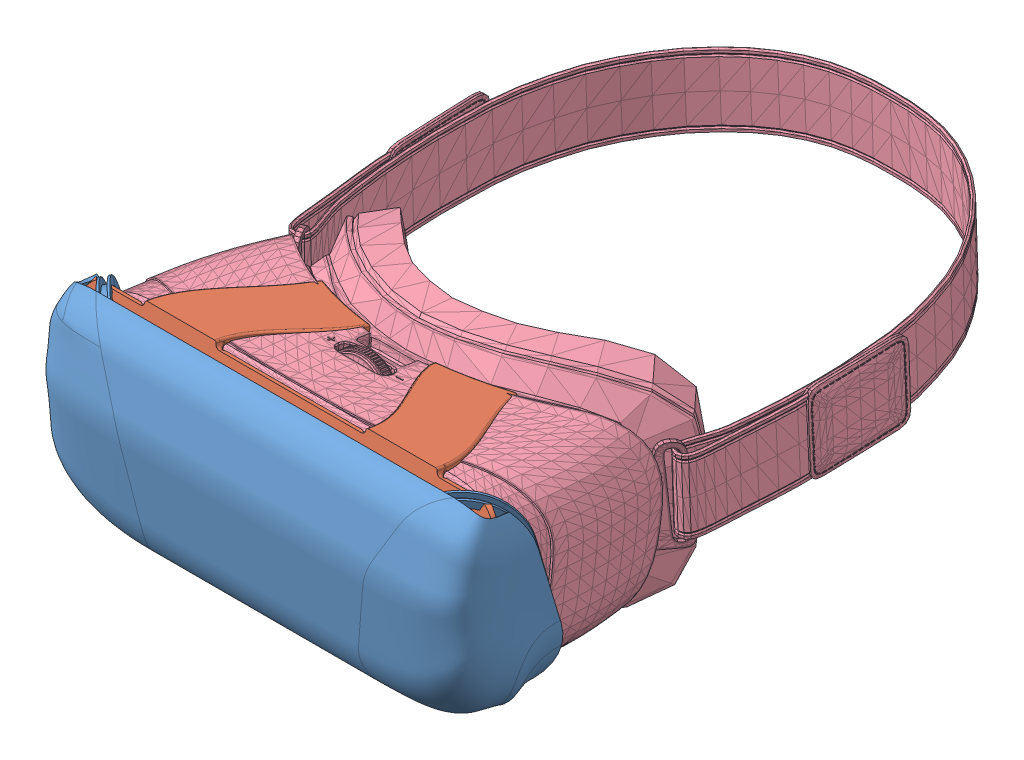
SolidWorks assembly 3coil_assem, configuration Default. Lengths in mm.
Overall size (227.31 162.97 341.93).
5 component instances, 5 part files, 7 mates.
Components (placement in the parent):
- coils-1: coils [Default] at (6.3911 53.5373 67.4612) x (1 0 0) z (0 0.069756 0.997564) size (229.11 102.7 66.76)
- Gear VR 2017_fix-1: Gear VR 2017_fix [Default] at origin (suppressed, hidden)
- case-1: case [Default] at (6.3911 95.712 57.18) x (1 0 0) z (0 0.173648 0.984808) size (213.62 98.27 76.29)
- electronics-1: electronics [Default] at (-28.0989 77.5708 62.4096) x (1 0 0) z (0 0.173648 0.984808) size (67.87 23.29 10)
- Gear VR 2017_surf_import-1: Gear VR 2017_surf_import [Default] at (6.3781 -8.2638 17.8982) x (1 0 0) z (0 0.139173 0.990268) size (217.03 119.93 317.65)
Mates (geometry in assembly coordinates):
- Coincident4: coincident: point of assembly; point of Gear VR 2017_fix-1; point of assembly
- Coincident5: coincident: plane of assembly; plane of assembly; plane of coils-1 through (112.1411 30.8384 60.3273) normal (1 0 0); plane of case-1 through (112.1411 96.0593 59.1496) normal (1 0 0)
- Coincident6: coincident: plane of assembly; plane of assembly; plane of coils-1 through (-99.3589 68.3817 62.5314) normal (0 0.190809 -0.981627); plane of case-1 through (-94.3589 72.4239 63.3172) normal (0 -0.190809 0.981627)
- Coincident7: coincident: plane of assembly; plane of assembly; plane of case-1 through (6.3911 96.0593 59.1496) normal (0 0.173648 0.984808); plane of electronics-1 through (-28.0989 77.5708 62.4096) normal (0 -0.173648 -0.984808)
- Coincident8: coincident: plane of assembly; plane of assembly; plane of case-1 through (-28.0989 63.5349 -17.1921) normal (1 0 0); plane of electronics-1 through (-28.0989 79.3073 72.2577) normal (-1 0 0)
- Coincident9: coincident: plane of assembly; plane of assembly; plane of case-1 through (-28.0989 63.5349 -17.1921) normal (0 -0.984808 0.173648); plane of electronics-1 through (-28.0989 79.3073 72.2577) normal (0 0.984808 -0.173648)
- Coincident10: coincident: unknown of case-1; unknown of ?
